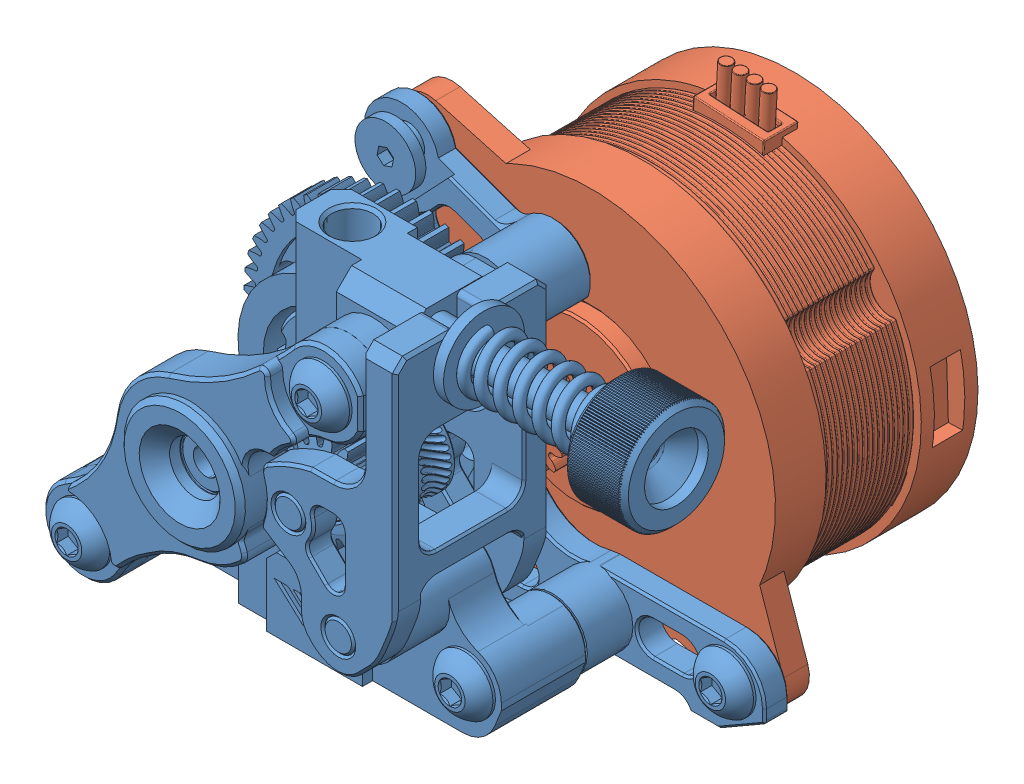
SolidWorks assembly ASM_MA_Extruder_V1, configuration Default. Lengths in mm.
Overall size (62.49 57.22 45.42).
2 component instances, 2 part files, 2 mates.
Components (placement in the parent):
- PRT_MA_VZ_Hextrudort-2: PRT_MA_VZ_Hextrudort [Default] at (16.116 12.2179 40.659) x (1 0 0) z (0 1 0) size (55.08 29 38.4)
- PRT_MA_LDO_20mm_Nema14-1: PRT_MA_LDO_20mm_Nema14 [Default] at (-5.0462 48.6582 8.2878) x (-0.88148 0.472221 -0.000518) z (0.000441 -0.000274 -1) size (48.79 38.77 26.01)
Mates (geometry in assembly coordinates):
- Coincident1: coincident anti-aligned: plane of PRT_MA_VZ_Hextrudort-2 through (25.2677 36.754 28.109) normal (0 0 -1); plane of PRT_MA_LDO_20mm_Nema14-1 through (27.0635 31.5061 28.109) normal (0 0 1)
- Slot2: slot aligned: cylinder of PRT_MA_LDO_20mm_Nema14-1 through (10.9114 46.6626 28.109) axis (0 0 -1) radius 3; cylinder of PRT_MA_VZ_Hextrudort-2 through (10.9114 46.6626 31.259) axis (0 0 -1) radius 1.6; cylinder of PRT_MA_VZ_Hextrudort-2 through (9.5762 45.1736 31.259) axis (0 0 -1) radius 1.6
